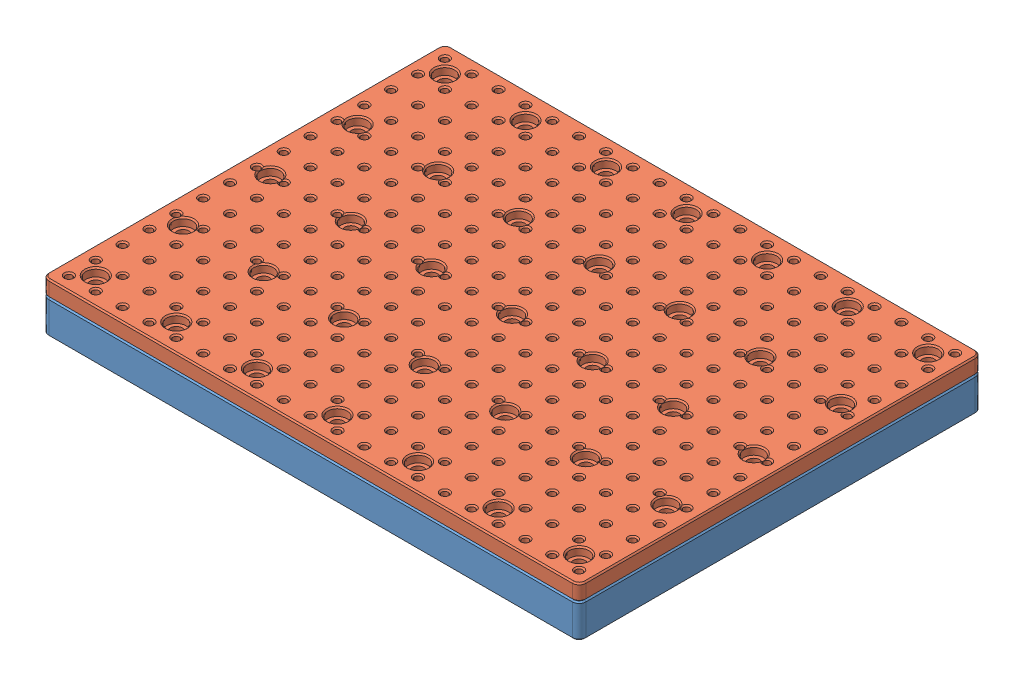
SolidWorks assembly Y_axis_rollere, configuration Default. Lengths in mm.
Overall size (400 37.42 300).
32 component instances, 7 part files, 19 mates.
Components (placement in the parent):
- HGH20CAZ0C-1: HGH20CAZ0C [Default] at (-147.4668 15.9869 125.7613) size (44 25.5 89.06) (hidden)
  - HGH20CAZ0C, BLOCK, MIDSECTION-2: HGH20CAZ0C, BLOCK, MIDSECTION [Default] at origin size (44 25.5 77.5)
  - HGH20CAZ0C, BLOCK OIL FILLING PART-1: HGH20CAZ0C, BLOCK OIL FILLING PART [Default] at (0 11 33.75) x (0 0 -1) z (0 1 0) size (16.4 16.42 9.24)
  - HGH20CAZ0C, SCREW HEAD-1: HGH20CAZ0C, SCREW HEAD [Default] at (18.75 2.9 36.65) x (0 0 1) z (-1 0 0) size (2.26 5 5)
  - HGH20CAZ0C, SCREW HEAD-2: HGH20CAZ0C, SCREW HEAD [Default] at (-18.75 2.9 36.65) x (0 0 1) z (-1 0 0) size (2.26 5 5)
  - HGH20CAZ0C, SCREW HEAD-3: HGH20CAZ0C, SCREW HEAD [Default] at (18.75 2.9 -36.65) x (0 0 -1) z (1 0 0) size (2.26 5 5)
  - HGH20CAZ0C, SCREW HEAD-4: HGH20CAZ0C, SCREW HEAD [Default] at (-18.75 2.9 -36.65) x (0 0 -1) z (1 0 0) size (2.26 5 5)
- HGH20CAZ0C-2: HGH20CAZ0C [Default] at (52.5332 15.9869 125.7613) size (44 25.5 89.06) (hidden)
  - HGH20CAZ0C, BLOCK, MIDSECTION-2: HGH20CAZ0C, BLOCK, MIDSECTION [Default] at origin size (44 25.5 77.5)
  - HGH20CAZ0C, BLOCK OIL FILLING PART-1: HGH20CAZ0C, BLOCK OIL FILLING PART [Default] at (0 11 33.75) x (0 0 -1) z (0 1 0) size (16.4 16.42 9.24)
  - HGH20CAZ0C, SCREW HEAD-1: HGH20CAZ0C, SCREW HEAD [Default] at (18.75 2.9 36.65) x (0 0 1) z (-1 0 0) size (2.26 5 5)
  - HGH20CAZ0C, SCREW HEAD-2: HGH20CAZ0C, SCREW HEAD [Default] at (-18.75 2.9 36.65) x (0 0 1) z (-1 0 0) size (2.26 5 5)
  - HGH20CAZ0C, SCREW HEAD-3: HGH20CAZ0C, SCREW HEAD [Default] at (18.75 2.9 -36.65) x (0 0 -1) z (1 0 0) size (2.26 5 5)
  - HGH20CAZ0C, SCREW HEAD-4: HGH20CAZ0C, SCREW HEAD [Default] at (-18.75 2.9 -36.65) x (0 0 -1) z (1 0 0) size (2.26 5 5)
- HGH20CAZ0C-3: HGH20CAZ0C [Default] at (52.5332 15.9869 -19.7387) x (-1 0 0) z (0 0 -1) size (44 25.5 89.06) (hidden)
  - HGH20CAZ0C, BLOCK, MIDSECTION-2: HGH20CAZ0C, BLOCK, MIDSECTION [Default] at origin size (44 25.5 77.5)
  - HGH20CAZ0C, BLOCK OIL FILLING PART-1: HGH20CAZ0C, BLOCK OIL FILLING PART [Default] at (0 11 33.75) x (0 0 -1) z (0 1 0) size (16.4 16.42 9.24)
  - HGH20CAZ0C, SCREW HEAD-1: HGH20CAZ0C, SCREW HEAD [Default] at (18.75 2.9 36.65) x (0 0 1) z (-1 0 0) size (2.26 5 5)
  - HGH20CAZ0C, SCREW HEAD-2: HGH20CAZ0C, SCREW HEAD [Default] at (-18.75 2.9 36.65) x (0 0 1) z (-1 0 0) size (2.26 5 5)
  - HGH20CAZ0C, SCREW HEAD-3: HGH20CAZ0C, SCREW HEAD [Default] at (18.75 2.9 -36.65) x (0 0 -1) z (1 0 0) size (2.26 5 5)
  - HGH20CAZ0C, SCREW HEAD-4: HGH20CAZ0C, SCREW HEAD [Default] at (-18.75 2.9 -36.65) x (0 0 -1) z (1 0 0) size (2.26 5 5)
- HGH20CAZ0C-4: HGH20CAZ0C [Default] at (-147.4668 15.9869 -19.7387) x (-1 0 0) z (0 0 -1) size (44 25.5 89.06) (hidden)
  - HGH20CAZ0C, BLOCK, MIDSECTION-2: HGH20CAZ0C, BLOCK, MIDSECTION [Default] at origin size (44 25.5 77.5)
  - HGH20CAZ0C, BLOCK OIL FILLING PART-1: HGH20CAZ0C, BLOCK OIL FILLING PART [Default] at (0 11 33.75) x (0 0 -1) z (0 1 0) size (16.4 16.42 9.24)
  - HGH20CAZ0C, SCREW HEAD-1: HGH20CAZ0C, SCREW HEAD [Default] at (18.75 2.9 36.65) x (0 0 1) z (-1 0 0) size (2.26 5 5)
  - HGH20CAZ0C, SCREW HEAD-2: HGH20CAZ0C, SCREW HEAD [Default] at (-18.75 2.9 36.65) x (0 0 1) z (-1 0 0) size (2.26 5 5)
  - HGH20CAZ0C, SCREW HEAD-3: HGH20CAZ0C, SCREW HEAD [Default] at (18.75 2.9 -36.65) x (0 0 -1) z (1 0 0) size (2.26 5 5)
  - HGH20CAZ0C, SCREW HEAD-4: HGH20CAZ0C, SCREW HEAD [Default] at (-18.75 2.9 -36.65) x (0 0 -1) z (1 0 0) size (2.26 5 5)
- Y_Plate-1: Y_Plate [Default] at (-47.4668 31.9869 53.0113) x (1 0 0) z (0 1 0) size (400 300 25)
- Y_Fixture_Plate-1: Y_Fixture_Plate [Default] at (-47.4668 56.9869 53.0113) x (1 0 0) z (0 1 0) size (400 300 12.42)
- DSG16H Ball Nut Housing-2: DSG16H Ball Nut Housing [Default] at (-47.4668 7.9869 83.0113) x (1 0 0) z (0 1 0) size (52 40 40) (hidden)
- Nut_block_spacer-1: Nut_block_spacer [Default] at (-47.4668 27.9869 83.0113) x (1 0 0) z (0 1 0) size (52 40 4) (hidden)
Mates (geometry in assembly coordinates):
- Coincident12: coincident anti-aligned: plane of HGH20CAZ0C-3/HGH20CAZ0C, BLOCK, MIDSECTION-1 through (73.5332 31.9869 -44.9887) normal (0 1 0); plane of Y_Plate-1 through (-47.4668 31.9869 53.0113) normal (0 -1 0)
- Coincident13: coincident anti-aligned: plane of Y_Plate-1 through (-47.4668 56.9869 53.0113) normal (0 1 0); plane of Y_Fixture_Plate-1 through (-47.4668 56.9869 53.0113) normal (0 -1 0)
- Coincident14: coincident aligned: plane of Y_Plate-1 through (152.5332 56.9869 -96.9887) normal (1 0 0); plane of Y_Fixture_Plate-1 through (152.5332 68.9869 -96.9887) normal (1 0 0)
- Coincident15: coincident aligned: plane of Y_Plate-1 through (-247.4668 56.9869 203.0113) normal (0 0 1); plane of Y_Fixture_Plate-1 through (-247.4668 68.9869 203.0113) normal (0 0 1)
- Concentric1: concentric aligned: cylinder of HGH20CAZ0C-3/HGH20CAZ0C, BLOCK, MIDSECTION-2 through (68.5332 31.9869 -37.7387) axis (0 1 0) radius 2.1; cylinder of Y_Plate-1 through (68.5332 56.9869 -37.7387) axis (0 1 0) radius 2.75
- Concentric2: concentric aligned: cylinder of HGH20CAZ0C-3/HGH20CAZ0C, BLOCK, MIDSECTION-2 through (36.5332 31.9869 -1.7387) axis (0 1 0) radius 2.1; cylinder of Y_Plate-1 through (36.5332 56.9869 -1.7387) axis (0 1 0) radius 2.75
- Concentric4: concentric aligned: cylinder of HGH20CAZ0C-2/HGH20CAZ0C, BLOCK, MIDSECTION-2 through (68.5332 31.9869 107.7613) axis (0 1 0) radius 2.1; cylinder of Y_Plate-1 through (68.5332 56.9869 107.7613) axis (0 1 0) radius 2.75
- Concentric5: concentric aligned: cylinder of HGH20CAZ0C-2/HGH20CAZ0C, BLOCK, MIDSECTION-2 through (36.5332 31.9869 143.7613) axis (0 1 0) radius 2.1; cylinder of Y_Plate-1 through (36.5332 56.9869 143.7613) axis (0 1 0) radius 2.75
- Concentric6: concentric aligned: cylinder of HGH20CAZ0C-1/HGH20CAZ0C, BLOCK, MIDSECTION-2 through (-163.4668 31.9869 143.7613) axis (0 1 0) radius 2.1; cylinder of Y_Plate-1 through (-163.4668 56.9869 143.7613) axis (0 1 0) radius 2.75
- Concentric7: concentric aligned: cylinder of HGH20CAZ0C-1/HGH20CAZ0C, BLOCK, MIDSECTION-2 through (-131.4668 31.9869 107.7613) axis (0 1 0) radius 2.1; cylinder of Y_Plate-1 through (-131.4668 56.9869 107.7613) axis (0 1 0) radius 2.75
- Concentric8: concentric aligned: cylinder of HGH20CAZ0C-4/HGH20CAZ0C, BLOCK, MIDSECTION-2 through (-163.4668 31.9869 -37.7387) axis (0 1 0) radius 2.1; cylinder of Y_Plate-1 through (-163.4668 56.9869 -37.7387) axis (0 1 0) radius 2.75
- Concentric9: concentric aligned: cylinder of HGH20CAZ0C-4/HGH20CAZ0C, BLOCK, MIDSECTION-2 through (-131.4668 31.9869 -1.7387) axis (0 1 0) radius 2.1; cylinder of Y_Plate-1 through (-131.4668 56.9869 -1.7387) axis (0 1 0) radius 2.75
- Coincident17: coincident anti-aligned: plane of HGH20CAZ0C-4/HGH20CAZ0C, BLOCK, MIDSECTION-2 through (-168.4668 31.9869 -44.9887) normal (0 1 0); plane of Y_Plate-1 through (-47.4668 31.9869 53.0113) normal (0 -1 0)
- Coincident18: coincident anti-aligned: plane of HGH20CAZ0C-1/HGH20CAZ0C, BLOCK, MIDSECTION-2 through (-168.4668 31.9869 151.0113) normal (0 1 0); plane of Y_Plate-1 through (-47.4668 31.9869 53.0113) normal (0 -1 0)
- Coincident19: coincident anti-aligned: plane of HGH20CAZ0C-2/HGH20CAZ0C, BLOCK, MIDSECTION-2 through (31.5332 31.9869 151.0113) normal (0 1 0); plane of Y_Plate-1 through (-47.4668 31.9869 53.0113) normal (0 -1 0)
- InPlace1: in place: plane of DSG16H Ball Nut Housing-2 through (-73.4668 27.9869 83.0113) normal (0 1 0); plane of ? through (0 27.9869 0) normal (0 1 0); moOrthogonalPlaneRef_w of DSG16H Ball Nut Housing-2 through (-73.4668 27.9869 83.0113) normal (0 1 0); plane of ? through (0 27.9869 0) normal (0 0 -1); plane of DSG16H Ball Nut Housing-2 through (-73.4668 27.9869 83.0113) normal (0 1 0); plane of ? through (0 27.9869 0) normal (1 0 0); plane of DSG16H Ball Nut Housing-2 through (-73.4668 27.9869 83.0113) normal (0 1 0); unknown of Nut_block_spacer-1
- Coincident21: coincident aligned: plane of DSG16H Ball Nut Housing-2; plane of Nut_block_spacer-1
- Coincident22: coincident aligned: moOrthogonalPlaneRef_w of DSG16H Ball Nut Housing-2 through (-47.4668 27.9869 83.0113) normal (0 0 -1); plane of Nut_block_spacer-1 through (-47.4668 27.9869 83.0113) normal (0 0 -1)
- Coincident23: coincident anti-aligned: moOrthogonalPlaneRef_w of DSG16H Ball Nut Housing-2 through (-47.4668 27.9869 83.0113) normal (-1 0 0); plane of Nut_block_spacer-1 through (-47.4668 27.9869 83.0113) normal (1 0 0)
